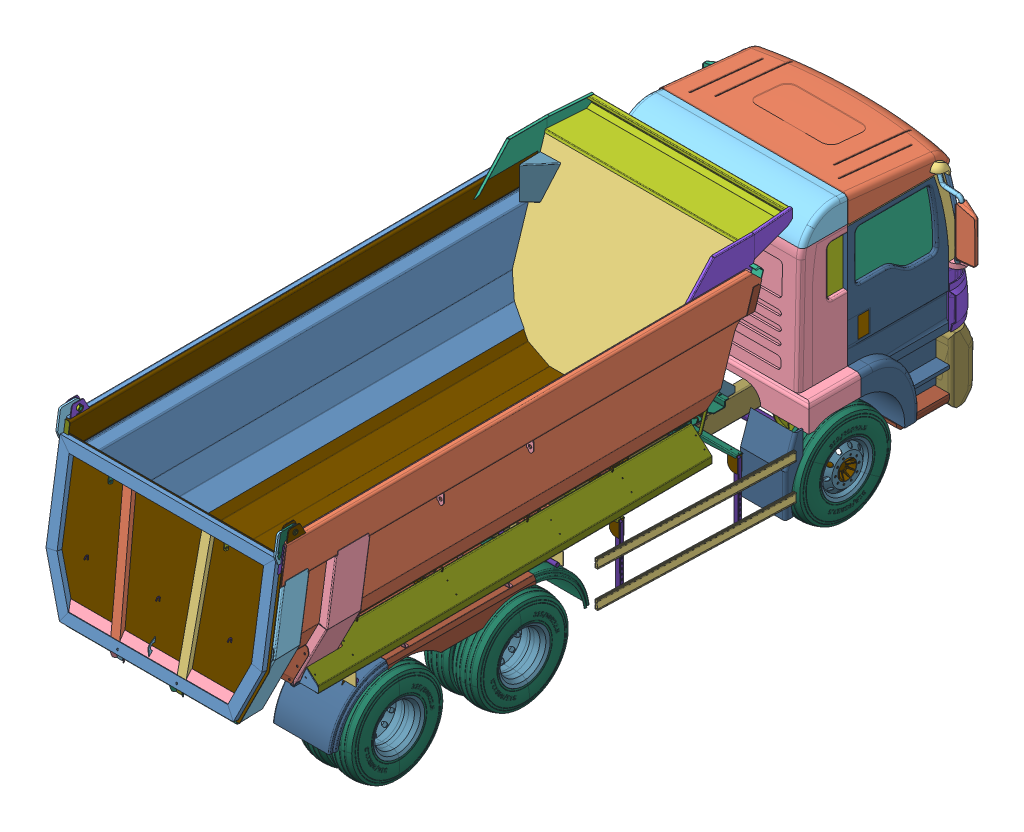
SolidWorks assembly MAN5, configuration Default. Lengths in mm. (continued)
Components (placement in the parent): (continued)
- MAN5.IGS-1: MAN5.IGS [Default] at origin size (3197.79 4674.46 9356.54) (continued)
  - Aynalama33360_pulll.IGS-9: Aynalama33360_pulll.IGS [Default] at (-450.3476 1324.558 3301.5348) x (-0.95234 0 -0.30504) z (0 -1 0) size (40 76.01 3.01)
  - Aynalama33360_pulll.IGS-10: Aynalama33360_pulll.IGS [Default] at (-450.3476 1352.558 3301.5348) x (-0.995286 0 0.096983) z (0 -1 0) size (40 76.01 3.01)
  - Aynalama33360_pulll.IGS-11: Aynalama33360_pulll.IGS [Default] at (-444.4001 1395.558 3378.3048) x (0.404503 0 -0.914537) z (0 -1 0) size (40 76.01 3.01)
  - Aynalama33360_pulll.IGS-12: Aynalama33360_pulll.IGS [Default] at (-450.3476 1395.558 3301.5348) x (0.404503 0 -0.914537) z (0 -1 0) size (40 76.01 3.01)
  - Aynalama33360_esnek baglanti poliuretan takoz.IGS-1: Aynalama33360_esnek baglanti poliuretan takoz.IGS [Default] at (-479.517 1445.558 2461.1366) x (0.305771 0 -0.952105) z (-0.952105 0 -0.305771) size (40.39 40.39 40.78)
  - Aynalama33360_esnek baglanti poliuretan takoz.IGS-2: Aynalama33360_esnek baglanti poliuretan takoz.IGS [Default] at (-479.517 1445.558 2381.1366) x (0.305771 0 -0.952105) z (-0.952105 0 -0.305771) size (40.39 40.39 40.78)
  - Aynalama33360_HEX NUT - ISO 8673 - M16 X 1.5.IGS-1: Aynalama33360_HEX NUT - ISO 8673 - M16 X 1.5.IGS [Default] at (-479.517 1463.358 2461.1366) x (0 -1 0) z (-0.270173 0 -0.962812) size (15.03 27.75 27.75)
  - Aynalama33360_HEX NUT - ISO 8673 - M16 X 1.5.IGS-2: Aynalama33360_HEX NUT - ISO 8673 - M16 X 1.5.IGS [Default] at (-479.517 1463.358 2381.1366) x (0 -1 0) z (-0.270173 0 -0.962812) size (15.03 27.75 27.75)
  - Aynalama33360_HEX NUT - ISO 8673 - M16 X 1.5.IGS-3: Aynalama33360_HEX NUT - ISO 8673 - M16 X 1.5.IGS [Default] at (-444.4001 1413.358 3378.3048) x (0 -1 0) z (0.336021 0 -0.941854) size (15.03 27.75 27.75)
  - Aynalama33360_HEX NUT - ISO 8673 - M16 X 1.5.IGS-4: Aynalama33360_HEX NUT - ISO 8673 - M16 X 1.5.IGS [Default] at (-450.3476 1413.358 3301.5348) x (0 -1 0) z (0.336021 0 -0.941854) size (15.03 27.75 27.75)
  - Aynalama33360_MS 008.IGS-1: Aynalama33360_MS 008.IGS [Default] at (-609.242 1337.558 3134.9181) x (0.077241 0 0.997012) z (0 1 0) size (151.36 57.01 58.73)
  - Aynalama33360_MS 009.IGS-1: Aynalama33360_MS 009.IGS [Default] at (-439.052 1337.558 3121.7331) x (-0.077241 0 -0.997012) z (-0.997012 0 0.077241) size (152.03 59.04 8.35)
  - Aynalama33360_burçlu baðlantý burcu.IGS-1: Aynalama33360_burçlu baðlantý burcu.IGS [Default] at (-444.4001 1355.558 3378.3048) x (0.984937 0 0.172914) z (0 -1 0) size (42 42 40.39)
  - Aynalama33360_burçlu baðlantý burcu.IGS-2: Aynalama33360_burçlu baðlantý burcu.IGS [Default] at (-450.3476 1355.558 3301.5348) x (0.984937 0 0.172914) z (0 -1 0) size (42 42 40.39)
  - AynalamaSon_model_3.IGS-1: AynalamaSon_model_3.IGS [Default] at (-365.1668 1272.558 4408.28) x (0 0 -1) z (1 0 0) size (155.01 200.01 10.01)
  - AynalamaSon_model_3.IGS-2: AynalamaSon_model_3.IGS [Default] at (-365.1668 1272.558 5438.28) x (0 0 -1) z (1 0 0) size (155.01 200.01 10.01)
  - AynalamaSon_model_3.IGS-3: AynalamaSon_model_3.IGS [Default] at (-365.1668 1272.558 6138.28) x (0 0 -1) z (1 0 0) size (155.01 200.01 10.01)
  - Aynalama33360_arkamilbaðlantý.IGS-1: Aynalama33360_arkamilbaðlantý.IGS [Default] at (-365.1668 311.3597 8865.1072) x (0 0 -1) z (1 0 0) size (490.66 250.98 10.19)
  - Ayak U þase parçasý.IGS-1: Ayak U þase parçasý.IGS [Default] at (-372.5244 1364.558 6412.1883) x (1 0 0) z (0 1 0) size (60.01 150.01 180.01)
  - Ayak U þase parçasý.IGS-2: Ayak U þase parçasý.IGS [Default] at (-372.5244 1364.558 5250.1883) x (1 0 0) z (0 1 0) size (60.01 150.01 180.01)
  - ayakl flans.IGS-1: ayakl flans.IGS [Default] at (-415.1668 1481.9529 6462.5787) x (0 0 -1) z (1 0 0) size (125.01 130.01 8.01)
  - ayakl flans.IGS-2: ayakl flans.IGS [Default] at (-415.1668 1481.9529 5300.5787) x (0 0 -1) z (1 0 0) size (125.01 130.01 8.01)
  - Üst kapama L ayak sasi parçasý 21.IGS-1: Üst kapama L ayak sasi parçasý 21.IGS [Default] at (-423.1668 1470.1164 6419.9663) x (0 0 1) z (-1 0 0) size (70.01 70.39 760.39)
  - Üst kapama L ayak sasi parçasý 21.IGS-2: Üst kapama L ayak sasi parçasý 21.IGS [Default] at (-423.1668 1470.1164 5257.9663) x (0 0 1) z (-1 0 0) size (70.01 70.39 760.39)
  - Plastik çamurluk üst kapama1.IGS-1: Plastik çamurluk üst kapama1.IGS [Default] at (-520.1668 1374.558 6658.78) x (-1 0 0) z (0 0 -1) size (690.02 215.03 1650.01)
  - YAPI_plastik camurluk.IGS-1: YAPI_plastik camurluk.IGS [Default] at (-530.1668 -54790.0929 231516.4576) x (0 0.148915 -0.98885) z (1 0 0) size (762.44 555.79 670.01)
  - YAPI_boruu.IGS-1: YAPI_boruu.IGS [Default] at (-355.1668 1394.078 6953.9165) x (0 0.37163 0.928381) z (-1 0 0) size (42.01 42.01 802.01)
  - YAPI_plastik cmurluk bru ust bayrak.IGS-1: YAPI_plastik cmurluk bru ust bayrak.IGS [Default] at (-1051.5754 -129957.1173 197509.9483) x (0 0.487288 -0.873241) z (1 0 0) size (168.01 58.89 5.62)
  - YAPI_plastik cmurluk bru ust bayrak.IGS-2: YAPI_plastik cmurluk bru ust bayrak.IGS [Default] at (-751.5754 -129957.1173 197509.9483) x (0 0.487288 -0.873241) z (1 0 0) size (168.01 58.89 5.62)
  - AynalamaYAPI_boruu.IGS-1: AynalamaYAPI_boruu.IGS [Default] at (-355.1668 1394.078 4713.6435) x (0 0.37163 -0.928381) z (1 0 0) size (42.01 42.01 802.01)
  - AynalamaYAPI_boruu.IGS-2: AynalamaYAPI_boruu.IGS [Default] at (406.8332 1394.078 6953.9165) x (0 0.37163 0.928381) z (-1 0 0) size (42.01 42.01 802.01)
  - AynalamaYAPI_plastik cmurluk bru ust bayrak.IGS-1: AynalamaYAPI_plastik cmurluk bru ust bayrak.IGS [Default] at (-1051.5754 -129957.1173 -185842.3882) x (0 0.487288 0.873241) z (-1 0 0) size (168.01 58.28 5.3)
  - AynalamaYAPI_plastik cmurluk bru ust bayrak.IGS-2: AynalamaYAPI_plastik cmurluk bru ust bayrak.IGS [Default] at (-751.5754 -129957.1173 -185842.3882) x (0 0.487288 0.873241) z (-1 0 0) size (168.01 58.28 5.3)
  - AynalamaYAPI_plastik cmurluk bru ust bayrak.IGS-3: AynalamaYAPI_plastik cmurluk bru ust bayrak.IGS [Default] at (803.2418 -129957.1173 197509.9483) x (0 0.487288 -0.873241) z (1 0 0) size (168.01 58.28 5.3)
  - AynalamaYAPI_plastik cmurluk bru ust bayrak.IGS-4: AynalamaYAPI_plastik cmurluk bru ust bayrak.IGS [Default] at (1103.2418 -129957.1173 197509.9483) x (0 0.487288 -0.873241) z (1 0 0) size (168.01 58.28 5.3)
  - AynalamaYAPI_plastik camurluk.IGS-1: AynalamaYAPI_plastik camurluk.IGS [Default] at (-530.1668 -54790.0929 -219848.8976) x (0 0.148915 0.98885) z (-1 0 0) size (762.44 554.71 670.01)
  - AynalamaYAPI_plastik camurluk.IGS-2: AynalamaYAPI_plastik camurluk.IGS [Default] at (581.8332 -54790.0929 231516.4576) x (0 0.148915 -0.98885) z (1 0 0) size (762.44 554.71 670.01)
  - AynalamaPlastik çamurluk üst kapama1.IGS-1: AynalamaPlastik çamurluk üst kapama1.IGS [Default] at (571.8332 1374.558 6658.78) size (690.02 215.03 1650.01)
  - Aynalamaayakl flans.IGS-1: Aynalamaayakl flans.IGS [Default] at (466.8332 1481.9529 6462.5787) x (0 0 -1) z (1 0 0) size (125.01 130.01 8.01)
  - Aynalamaayakl flans.IGS-2: Aynalamaayakl flans.IGS [Default] at (466.8332 1481.9529 5300.5787) x (0 0 -1) z (1 0 0) size (125.01 130.01 8.01)
  - AynalamaÜst kapama L ayak sasi parçasý 21.IGS-1: AynalamaÜst kapama L ayak sasi parçasý 21.IGS [Default] at (474.8332 1470.1164 6419.9663) x (0 0 1) z (-1 0 0) size (70.01 70.39 760.39)
  - AynalamaÜst kapama L ayak sasi parçasý 21.IGS-2: AynalamaÜst kapama L ayak sasi parçasý 21.IGS [Default] at (474.8332 1470.1164 5257.9663) x (0 0 1) z (-1 0 0) size (70.01 70.39 760.39)
  - AynalamaAyak U þase parçasý.IGS-1: AynalamaAyak U þase parçasý.IGS [Default] at (424.1908 1364.558 6412.1883) x (-1 0 0) z (0 -1 0) size (60.01 150.01 180.01)
  - AynalamaAyak U þase parçasý.IGS-2: AynalamaAyak U þase parçasý.IGS [Default] at (424.1908 1364.558 5250.1883) x (-1 0 0) z (0 -1 0) size (60.01 150.01 180.01)
  - AynalamaAynalamaYAPI_plastik camurluk.IGS-1: AynalamaAynalamaYAPI_plastik camurluk.IGS [Default] at (581.8332 -54790.0929 -219848.8976) x (0 0.148915 0.98885) z (-1 0 0) size (762.44 555.79 670.01)
  - AynalamaAynalamaYAPI_plastik cmurluk bru ust bayrak.IGS-1: AynalamaAynalamaYAPI_plastik cmurluk bru ust bayrak.IGS [Default] at (803.2418 -129957.1173 -185842.3882) x (0 0.487288 0.873241) z (-1 0 0) size (168.01 58.89 5.62)
  - AynalamaAynalamaYAPI_plastik cmurluk bru ust bayrak.IGS-2: AynalamaAynalamaYAPI_plastik cmurluk bru ust bayrak.IGS [Default] at (1103.2418 -129957.1173 -185842.3882) x (0 0.487288 0.873241) z (-1 0 0) size (168.01 58.89 5.62)
  - AynalamaAynalamaYAPI_boruu.IGS-1: AynalamaAynalamaYAPI_boruu.IGS [Default] at (406.8332 1394.078 4713.6435) x (0 0.37163 -0.928381) z (1 0 0) size (42.01 42.01 802.01)
  - M5 - erp33360_TABAN 8 MM ST.IGS-1: M5 - erp33360_TABAN 8 MM ST.IGS [Default] at (2711.0125 794.7914 10334.4906) x (-1 0 0) z (0 0.005539 -0.999985) size (1888.79 207.2 5094.21)
  - M5 - erp33360_YAN 6 MM ST.IGS-1: M5 - erp33360_YAN 6 MM ST.IGS [Default] at (-3149.2259 1030.8858 2339.3517) x (1 0 0) z (0 -0.005539 0.999985) size (345.97 1417.88 5529.51)
  - M5 - erp33360_MirrorYAN 6 MM ST.IGS-1: M5 - erp33360_MirrorYAN 6 MM ST.IGS [Default] at (-555.1726 1030.8858 2339.3517) x (1 0 0) z (0 -0.005539 0.999985) size (345.97 1417.88 5529.51)
  - M5 - erp33360_ÖNPANEL 6 MM ST.IGS-1: M5 - erp33360_ÖNPANEL 6 MM ST.IGS [Default] at (3482.8014 -1032.9201 3905.3475) x (-1 0 0) z (0 -0.303745 -0.952753) size (2308.01 1803.01 6.01)
  - M5 - erp33360_ÖZBEKÝSTAN kulak krosu.IGS-1: M5 - erp33360_ÖZBEKÝSTAN kulak krosu.IGS [Default] at (1008.3381 57456.9661 -197352.5561) x (0 -0.005539 0.999985) z (-1 0 0) size (380.01 85.01 1965.01)
  - M5 - erp33360_ÖZBEKÝSTAN Büyük Yan Kros.IGS-1: M5 - erp33360_ÖZBEKÝSTAN Büyük Yan Kros.IGS [Default] at (-1441.0535 2620.6295 10762.7624) x (0.390684 -0.920485 0.00854) z (-0.920505 -0.39072 -0.00295) size (1326.04 856.53 453.89)
  - M5 - erp33360_ÖZBEKÝSTAN En Arka Taban Krosu.IGS-1: M5 - erp33360_ÖZBEKÝSTAN En Arka Taban Krosu.IGS [Default] at (1075.8381 60014.1611 -302542.0948) x (0 -0.005539 0.999985) z (-1 0 0) size (149.44 170.01 1920.62)
  - M5 - erp33360_ÖZBEKÝSTAN küçük yan kros.IGS-1: M5 - erp33360_ÖZBEKÝSTAN küçük yan kros.IGS [Default] at (-1242.2043 1026.8349 7834.3506) x (0 0.150962 0.98854) z (0 0.98854 -0.150962) size (819.28 418.27 1464.92)
  - M5 - erp33360_HD_601.IGS-1: M5 - erp33360_HD_601.IGS [Default] at (25.8154 3173.364 2552.8076) x (1 -0.000135 0.000043) z (0.000141 0.952753 -0.303745) size (240.01 5.01 319.27)
  - M5 - erp33360_HD_602.IGS-1: M5 - erp33360_HD_602.IGS [Default] at (21.8458 3335.9395 2354.6947) x (-0.000135 -0.999999 -0.001661) z (1 -0.000135 0.000043) size (8.01 308.36 252.01)
  - M5 - erp33360_KMK 214.IGS-1: M5 - erp33360_KMK 214.IGS [Default] at (-94.1776 3178.3559 2403.4311) x (-0.000135 -0.999999 -0.001661) z (1 -0.000135 0.000043) size (302.82 405.21 6.16)
  - M5 - erp33360_KMK 214.IGS-2: M5 - erp33360_KMK 214.IGS [Default] at (151.8224 3178.3227 2403.4417) x (-0.000135 -0.999999 -0.001661) z (1 -0.000135 0.000043) size (302.82 405.21 6.16)
  - M5 - erp33360_HD_604.IGS-1: M5 - erp33360_HD_604.IGS [Default] at (-16.9955 -12880.7962 5963.2245) x (-0.000135 -0.999959 0.009015) z (1 -0.000135 0.000043) size (157.84 185.04 79.51)
  - M5 - erp33360_HD_604.IGS-2: M5 - erp33360_HD_604.IGS [Default] at (143.5045 -12880.8178 5963.2314) x (-0.000135 -0.999959 0.009015) z (1 -0.000135 0.000043) size (157.84 185.04 79.51)
  - M5 - erp33360_KMK 213.IGS-1: M5 - erp33360_KMK 213.IGS [Default] at (-6.6689 3239.4117 2394.0646) x (0.000135 0.999992 0.003883) z (-1 0.000135 -0.000043) size (167.21 326.2 8.85)
  - M5 - erp33360_KMK 213.IGS-2: M5 - erp33360_KMK 213.IGS [Default] at (66.3311 3239.4018 2394.0677) x (0.000135 0.999992 0.003883) z (-1 0.000135 -0.000043) size (167.21 326.2 8.85)
  - M5 - erp33360_HDS_606.IGS-1: M5 - erp33360_HDS_606.IGS [Default] at (-44.6627 3267.742 2337.2221) x (-0.000007 0.253545 0.967324) z (1 -0.000135 0.000043) size (72.14 72 30.01)
  - M5 - erp33360_HDS_607.IGS-1: M5 - erp33360_HDS_607.IGS [Default] at (66.3373 3267.7271 2337.2269) x (-0.000135 -0.999999 -0.001661) z (1 -0.000135 0.000043) size (72 72 10.01)
  - M5 - erp33360_HDS_608.IGS-1: M5 - erp33360_HDS_608.IGS [Default] at (-50.6627 3267.7428 2337.2219) x (-0.000141 -0.967324 0.253545) z (1 -0.000135 0.000043) size (49 49.59 145.46)
  - M5 - erp33360_ÖZBEKÝSTAN ön dikme.IGS-1: M5 - erp33360_ÖZBEKÝSTAN ön dikme.IGS [Default] at (-168195.7295 -7372.7682 -32398.8379) x (1 0 0) z (0 -0.952753 0.303745) size (152.43 80.67 1836.48)
  - M5 - erp33360_ÖZBEKÝSTAN öngöðüs kuþak krosu.IGS-1: M5 - erp33360_ÖZBEKÝSTAN öngöðüs kuþak krosu.IGS [Default] at (-1218.0423 -352742.0932 105385.5445) x (0 0.953195 -0.302356) z (1 0 0) size (367.53 86.57 1008.59)
  - M5 - erp33360_iç kayýtr.IGS-1: M5 - erp33360_iç kayýtr.IGS [Default] at (-3031.6176 2222.8106 2486.7487) x (1 0 0) z (0 -0.005539 0.999985) size (71.18 295.53 5329.09)
  - M5 - erp33360_ÖZBEKÝSTAN kilit krosu bayrak.IGS-1: M5 - erp33360_ÖZBEKÝSTAN kilit krosu bayrak.IGS [Default] at (-4536.9786 -10452.359 13580.8312) x (1 0 0) z (0 0.430757 0.902468) size (617.2 521.07 142.75)
  - M5 - erp33360_ÖZBEKÝSTAN kilit takviye 2.IGS-1: M5 - erp33360_ÖZBEKÝSTAN kilit takviye 2.IGS [Default] at (-236.4961 1585.2287 7897.2862) x (1 0 0) z (0 -0.144581 -0.989493) size (437.72 186.93 142.51)
  - M5 - erp33360_MirrorÖZBEKÝSTAN ön dikme.IGS-1: M5 - erp33360_MirrorÖZBEKÝSTAN ön dikme.IGS [Default] at (164491.3309 -7373.2589 -32402.351) x (1 0 0) z (0 -0.952753 0.303745) size (152.47 80.67 1836.48)
  - M5 - erp33360_MirrorÖZBEKÝSTAN Büyük Yan Kros.IGS-1: M5 - erp33360_MirrorÖZBEKÝSTAN Büyük Yan Kros.IGS [Default] at (25.2904 -837.5574 10794.8351) x (0.390684 0.920485 -0.00854) z (0.920505 -0.39072 -0.00295) size (1326.07 873.47 448.36)
  - M5 - erp33360_AynalamaÖZBEKÝSTAN kilit krosu bayrak.IGS-1: M5 - erp33360_AynalamaÖZBEKÝSTAN kilit krosu bayrak.IGS [Default] at (4588.6547 -10452.359 13580.8312) x (-1 0 0) z (0 -0.430757 -0.902468) size (617.2 521.07 142.75)
  - M5 - erp33360_çamurluk sacý_k4.IGS-1: M5 - erp33360_çamurluk sacý_k4.IGS [Default] at (-3152.8435 697.3199 3027.2234) x (0.999992 0.00393 0.000022) z (0 -0.005539 0.999985) size (264.76 280.89 4405.19)
  - M5 - erp33360_ön çamurluk ayaðý_k6.IGS-1: M5 - erp33360_ön çamurluk ayaðý_k6.IGS [Default] at (-2993.8042 653.5355 3032.9809) x (0.999992 0.003934 0.000022) z (0 -0.005539 0.999985) size (508.17 269.14 291.41)
  - M5 - erp33360_iç çamurluk ayaðý_k6.IGS-1: M5 - erp33360_iç çamurluk ayaðý_k6.IGS [Default] at (-2594.5939 882.7123 5853.2935) x (0.999992 0.003934 0.000022) z (0 -0.005539 0.999985) size (492.87 198.39 270.05)
  - M5 - erp33360_iç çamurluk ayaðý_k6.IGS-2: M5 - erp33360_iç çamurluk ayaðý_k6.IGS [Default] at (-2594.5941 893.5402 3898.3234) x (0.999992 0.003934 0.000022) z (0 -0.005539 0.999985) size (492.87 198.39 270.05)
  - M5 - erp33360_arka çamurluk ayaðý_6mm.IGS-1: M5 - erp33360_arka çamurluk ayaðý_6mm.IGS [Default] at (-2965.4571 531.7536 7416.3737) x (0.999992 0.003934 0.000022) z (0 -0.005539 0.999985) size (216.15 187.55 190)
  - M5 - erp33360_iç çamurluk ayaðý_paspas gelenler__.IGS-1: M5 - erp33360_iç çamurluk ayaðý_paspas gelenler__.IGS [Default] at (-2594.5513 889.1528 4697.3114) x (0.999992 0.003934 0.000022) z (0 -0.005539 0.999985) size (492.87 225.4 270.05)
  - M5 - erp33360_iç çamurluk ayaðý_paspas gelenler__.IGS-2: M5 - erp33360_iç çamurluk ayaðý_paspas gelenler__.IGS [Default] at (-2594.5511 876.3532 7008.276) x (0.999992 0.003934 0.000022) z (0 -0.005539 0.999985) size (492.87 225.4 270.05)
  - M5 - erp33360_KMK 236.IGS-1: M5 - erp33360_KMK 236.IGS [Default] at (-21515.7908 1653.5699 -20713.8331) x (-1 0 0) z (0 -0.999985 -0.005539) size (250.01 390.01 12.01)
  - M5 - erp33360_KMS 202.IGS-1: M5 - erp33360_KMS 202.IGS [Default] at (-434.1619 1492.1837 7160.4219) x (0 -0.999985 -0.005539) z (0 -0.005539 0.999985) size (60.01 45.01 8.01)
  - M5 - erp33360_KMS 202.IGS-2: M5 - erp33360_KMS 202.IGS [Default] at (-434.1619 1490.9985 7374.4186) x (0 -0.999985 -0.005539) z (0 -0.005539 0.999985) size (60.01 45.01 8.01)
  - M5 - erp33360_KMS 202.IGS-3: M5 - erp33360_KMS 202.IGS [Default] at (-564.1619 1492.1394 7168.4218) x (0 -0.999985 -0.005539) z (0 0.005539 -0.999985) size (60.01 45.01 8.01)
  - M5 - erp33360_KMS 202.IGS-4: M5 - erp33360_KMS 202.IGS [Default] at (-564.1619 1490.9542 7382.4185) x (0 -0.999985 -0.005539) z (0 0.005539 -0.999985) size (60.01 45.01 8.01)
  - M5 - erp33360_HD 654.IGS-1: M5 - erp33360_HD 654.IGS [Default] at (-404.1619 1405.558 7270.78) x (-1 0 0) z (0 0.1474 -0.989077) size (171.89 100 100)
  - M5 - erp33360_KMK 226.IGS-1: M5 - erp33360_KMK 226.IGS [Default] at (-579.1619 1577.7689 7055.8305) x (0 -0.005539 0.999985) z (1 0 0) size (86.06 24.53 5.01)
  - M5 - erp33360_KMS 298.IGS-1: M5 - erp33360_KMS 298.IGS [Default] at (-564.1619 -80578.3775 132955.5354) x (0 -0.006857 0.999976) z (1 0 0) size (380.01 164.01 10.01)
  - M5 - erp33360_KMS 298.IGS-2: M5 - erp33360_KMS 298.IGS [Default] at (-444.1619 -80578.3775 132955.5354) x (0 -0.006857 0.999976) z (1 0 0) size (380.01 164.01 10.01)
  - M5 - erp33360_KMS 207.IGS-1: M5 - erp33360_KMS 207.IGS [Default] at (-554.1619 30316.5861 -13567.0822) x (0 0.005539 -0.999985) z (1 0 0) size (344.29 150.76 110.01)
  - M5 - erp33360_kros köþebent.IGS-1: M5 - erp33360_kros köþebent.IGS [Default] at (-937.9193 1507.0066 7461.4935) x (-0.390731 0.920493 0.004765) z (0.000854 0.005539 -0.999984) size (60.24 41.83 380.01)
  - M5 - erp33360_Aynalamaçamurluk ayaðý köþebenti_6mm.IGS-1: M5 - erp33360_Aynalamaçamurluk ayaðý köþebenti_6mm.IGS [Default] at (-3118.1274 743.529 5840.5224) x (1 0 0) z (0 -0.005539 0.999985) size (278.76 183.65 137.55)
  - M5 - erp33360_Aynalamaçamurluk ayaðý köþebenti_6mm.IGS-2: M5 - erp33360_Aynalamaçamurluk ayaðý köþebenti_6mm.IGS [Default] at (-3118.1274 749.9315 4684.5402) x (1 0 0) z (0 -0.005539 0.999985) size (278.76 183.65 137.55)
  - M5 - erp33360_Aynalamaçamurluk ayaðý köþebenti_6mm.IGS-3: M5 - erp33360_Aynalamaçamurluk ayaðý köþebenti_6mm.IGS [Default] at (-3118.1274 737.132 6995.5047) x (1 0 0) z (0 -0.005539 0.999985) size (278.76 183.65 137.55)
  - M5 - erp33360_Aynalamaçamurluk ayaðý köþebenti_6mm.IGS-4: M5 - erp33360_Aynalamaçamurluk ayaðý köþebenti_6mm.IGS [Default] at (-3118.1274 754.3568 3885.5524) x (1 0 0) z (0 -0.005539 0.999985) size (278.76 183.65 137.55)
  - M5 - erp33360_çamurluk ayaðý küçük köþebent 6mm.IGS-1: M5 - erp33360_çamurluk ayaðý küçük köþebent 6mm.IGS [Default] at (-998.8645 -778.8309 7396.4339) x (-0.39073 0.920491 0.005098) z (0.000724 0.005846 -0.999983) size (119.97 59.66 44.44)
  - M5 - erp33360_þase kaçmazý 6 mm.IGS-1: M5 - erp33360_þase kaçmazý 6 mm.IGS [Default] at (-2259.5031 543.4533 3492.8973) x (0.996972 0.000431 -0.077762) z (0.077763 -0.005522 0.996957) size (80.34 92.23 6.28)
  - M5 - erp33360_þase kaçmazý 6 mm.IGS-2: M5 - erp33360_þase kaçmazý 6 mm.IGS [Default] at (-2265.2576 543.8619 3419.1225) x (0.996972 0.000431 -0.077762) z (0.077763 -0.005522 0.996957) size (80.34 92.23 6.28)
  - M5 - erp33360_þase kaçmazý arka sacý_6mm.IGS-1: M5 - erp33360_þase kaçmazý arka sacý_6mm.IGS [Default] at (-2258.7255 543.3981 3502.8668) x (0.996972 0.000431 -0.077762) z (0.077763 -0.005522 0.996957) size (89.64 108.39 102.98)
  - M5 - erp33360_Aynalamaiç kayýtr.IGS-1: M5 - erp33360_Aynalamaiç kayýtr.IGS [Default] at (3083.2937 2222.8106 2486.7487) x (-1 0 0) z (0 0.005539 -0.999985) size (71.18 295.53 5329.09)
  - M5 - erp33360_çamurluk ayaðý köþebenti_6mm.IGS-1: M5 - erp33360_çamurluk ayaðý köþebenti_6mm.IGS [Default] at (-3118.1274 759.0424 3039.5654) x (1 0 0) z (0 -0.005539 0.999985) size (276.76 187.48 132.2)
  - M5 - erp33360_siperlik yan sacý.IGS-1: M5 - erp33360_siperlik yan sacý.IGS [Default] at (-1128.1619 2915.0348 3291.601) x (0 0.005539 -0.999985) z (1 0 0) size (1286.13 449.51 548.53)
  - M5 - erp33360_siperlik.IGS-1: M5 - erp33360_siperlik.IGS [Default] at (-1128.1619 3194.9843 2755.6366) x (0 0.005539 -0.999985) z (1 0 0) size (492.33 158.99 2308.01)
  - M5 - erp33360_Aynalamasiperlik yan sacý.IGS-1: M5 - erp33360_Aynalamasiperlik yan sacý.IGS [Default] at (1179.8381 2915.0348 3291.601) x (0 0.005539 -0.999985) z (1 0 0) size (1286.13 442.38 555.99)
  - M5 - erp33360_Ön arka çamurluk_Yeni Tip_k3.IGS-1: M5 - erp33360_Ön arka çamurluk_Yeni Tip_k3.IGS [Default] at (-597.7041 1563.9747 4685.8761) x (0 -0.005539 0.999985) z (-0.999995 -0.003098 -0.000017) size (3.1 205.01 600.01)
  - M5 - erp33360_Ön arka çamurluk_Yeni Tip_k3.IGS-2: M5 - erp33360_Ön arka çamurluk_Yeni Tip_k3.IGS [Default] at (-597.7039 1551.1751 6996.8407) x (0 -0.005539 0.999985) z (-0.999995 -0.003098 -0.000017) size (3.1 205.01 600.01)
  - M5 - erp33360_önpanel dýþköþe takviyesi.IGS-1: M5 - erp33360_önpanel dýþköþe takviyesi.IGS [Default] at (-1224.329 2619.4628 2447.6999) x (0 0.302356 0.953195) z (-1 0 0) size (89.64 267.98 79.8)
  - M5 - erp33360_Aynalamaönpanel dýþköþe takviyesi.IGS-1: M5 - erp33360_Aynalamaönpanel dýþköþe takviyesi.IGS [Default] at (1276.0051 2619.4628 2447.6999) x (0 0.302356 0.953195) z (-1 0 0) size (89.64 267.98 79.8)
  - M5 - erp33360_iç sehim takviyesi.IGS-1: M5 - erp33360_iç sehim takviyesi.IGS [Default] at (-384.1619 1408.1547 7304.7483) x (0 0.005539 -0.999985) z (1 0 0) size (146.01 77.01 820.01)
  - M5 - erp33360_iç sehim takviyesi.IGS-2: M5 - erp33360_iç sehim takviyesi.IGS [Default] at (435.8381 1408.529 7237.1701) x (0 -0.005539 0.999985) z (-1 0 0) size (146.01 77.01 820.01)
  - M5 - erp33360_önpanel içköþe takviyesi.IGS-1: M5 - erp33360_önpanel içköþe takviyesi.IGS [Default] at (1251.1068 2575.8808 2876.615) x (-0.69944 0.002869 -0.714686) z (0.714692 0.002808 -0.699434) size (328.95 380.59 175.4)
  - M5 - erpAynalama33360_önpanel içköþe takviyesi.IGS-1: M5 - erpAynalama33360_önpanel içköþe takviyesi.IGS [Default] at (-1199.4307 2575.8808 2876.615) x (0.69944 0.002869 -0.714686) z (0.714692 -0.002808 0.699434) size (328.95 380.59 181.53)
  - M5 - erp33360_siperlik lamasý.IGS-1: M5 - erp33360_siperlik lamasý.IGS [Default] at (-1128.1619 2713.3631 2659.0764) x (-1 0 0) z (0 -0.30377 -0.952745) size (29.96 171.79 4.01)
  - M5 - erpAynalama33360_çamurluk sacý_k4.IGS-1: M5 - erpAynalama33360_çamurluk sacý_k4.IGS [Default] at (3204.5196 697.3199 3027.2234) x (-0.999992 0.00393 0.000022) z (0 0.005539 -0.999985) size (264.76 280.89 4405.19)
  - M5 - erpAynalama33360_ön çamurluk ayaðý_k6.IGS-1: M5 - erpAynalama33360_ön çamurluk ayaðý_k6.IGS [Default] at (3045.4803 653.5355 3032.9809) x (-0.999992 0.003934 0.000022) z (0 0.005539 -0.999985) size (507.88 268.85 302.92)
  - M5 - erpAynalama33360_iç çamurluk ayaðý_k6.IGS-1: M5 - erpAynalama33360_iç çamurluk ayaðý_k6.IGS [Default] at (2646.27 882.7123 5853.2935) x (-0.999992 0.003934 0.000022) z (0 0.005539 -0.999985) size (492.69 198.39 258.62)
  - M5 - erpAynalama33360_iç çamurluk ayaðý_k6.IGS-2: M5 - erpAynalama33360_iç çamurluk ayaðý_k6.IGS [Default] at (2646.2702 893.5402 3898.3234) x (-0.999992 0.003934 0.000022) z (0 0.005539 -0.999985) size (492.69 198.39 258.62)
  - M5 - erpAynalama33360_arka çamurluk ayaðý_6mm.IGS-1: M5 - erpAynalama33360_arka çamurluk ayaðý_6mm.IGS [Default] at (3017.1332 531.7536 7416.3737) x (-0.999992 0.003934 0.000022) z (0 0.005539 -0.999985) size (216.15 187.26 178.81)
  - M5 - erpAynalama33360_iç çamurluk ayaðý_paspas gelenler__.IGS-1: M5 - erpAynalama33360_iç çamurluk ayaðý_paspas gelenler__.IGS [Default] at (2646.2274 889.1528 4697.3114) x (-0.999992 0.003934 0.000022) z (0 0.005539 -0.999985) size (492.69 225.4 258.62)
  - M5 - erpAynalama33360_iç çamurluk ayaðý_paspas gelenler__.IGS-2: M5 - erpAynalama33360_iç çamurluk ayaðý_paspas gelenler__.IGS [Default] at (2646.2272 876.3532 7008.276) x (-0.999992 0.003934 0.000022) z (0 0.005539 -0.999985) size (492.69 225.4 258.62)
  - M5 - erpAynalama33360_Ön arka çamurluk_Yeni Tip_k3.IGS-1: M5 - erpAynalama33360_Ön arka çamurluk_Yeni Tip_k3.IGS [Default] at (649.3802 1563.9747 4685.8761) x (0 -0.005539 0.999985) z (-0.999995 0.003098 0.000017) size (3.07 205.01 600.01)
  - M5 - erpAynalama33360_Ön arka çamurluk_Yeni Tip_k3.IGS-2: M5 - erpAynalama33360_Ön arka çamurluk_Yeni Tip_k3.IGS [Default] at (649.38 1551.1751 6996.8407) x (0 -0.005539 0.999985) z (-0.999995 0.003098 0.000017) size (3.07 205.01 600.01)
  - M5 - erpAynalama33360_KMK 236.IGS-1: M5 - erpAynalama33360_KMK 236.IGS [Default] at (21567.4669 1653.5699 -20713.8331) x (1 0 0) z (0 0.999985 0.005539) size (250.01 390.01 12.01)
  - M5 - erpAynalama33360_KMS 202.IGS-1: M5 - erpAynalama33360_KMS 202.IGS [Default] at (485.8381 1492.1837 7160.4219) x (0 -0.999985 -0.005539) z (0 0.005539 -0.999985) size (60.01 45.01 8.01)
  - M5 - erpAynalama33360_KMS 202.IGS-2: M5 - erpAynalama33360_KMS 202.IGS [Default] at (485.8381 1490.9985 7374.4186) x (0 -0.999985 -0.005539) z (0 0.005539 -0.999985) size (60.01 45.01 8.01)
  - M5 - erpAynalama33360_KMS 202.IGS-3: M5 - erpAynalama33360_KMS 202.IGS [Default] at (615.8381 1492.1394 7168.4218) x (0 -0.999985 -0.005539) z (0 -0.005539 0.999985) size (60.01 45.01 8.01)
  - M5 - erpAynalama33360_KMS 202.IGS-4: M5 - erpAynalama33360_KMS 202.IGS [Default] at (615.8381 1490.9542 7382.4185) x (0 -0.999985 -0.005539) z (0 -0.005539 0.999985) size (60.01 45.01 8.01)
  - M5 - erpAynalama33360_HD 654.IGS-1: M5 - erpAynalama33360_HD 654.IGS [Default] at (455.8381 1405.558 7270.78) x (1 0 0) z (0 -0.1474 0.989077) size (170.95 100 100)
  - M5 - erpAynalama33360_KMK 226.IGS-1: M5 - erpAynalama33360_KMK 226.IGS [Default] at (630.8381 1577.7689 7055.8305) x (0 -0.005539 0.999985) z (1 0 0) size (86.06 25.37 5.43)
  - M5 - erpAynalama33360_KMS 298.IGS-1: M5 - erpAynalama33360_KMS 298.IGS [Default] at (615.8381 -80578.3775 132955.5354) x (0 -0.006857 0.999976) z (1 0 0) size (380.01 164.44 10.44)
  - M5 - erpAynalama33360_KMS 298.IGS-2: M5 - erpAynalama33360_KMS 298.IGS [Default] at (495.8381 -80578.3775 132955.5354) x (0 -0.006857 0.999976) z (1 0 0) size (380.01 164.44 10.44)
  - M5 - erpAynalama33360_KMS 207.IGS-1: M5 - erpAynalama33360_KMS 207.IGS [Default] at (605.8381 30316.5861 -13567.0822) x (0 0.005539 -0.999985) z (1 0 0) size (344.29 150.76 110.01)
  - M5 - erpAynalama33360_kros köþebent.IGS-1: M5 - erpAynalama33360_kros köþebent.IGS [Default] at (989.5954 1507.0066 7461.4935) x (0.390731 0.920493 0.004765) z (0.000854 -0.005539 0.999984) size (60.24 41.83 380.01)
  - M5 - erpAynalama33360_Aynalamaçamurluk ayaðý köþebenti_6mm.IGS-1: M5 - erpAynalama33360_Aynalamaçamurluk ayaðý köþebenti_6mm.IGS [Default] at (3169.8035 743.529 5840.5224) x (-1 0 0) z (0 0.005539 -0.999985) size (278.95 183.65 132.2)
  - M5 - erpAynalama33360_Aynalamaçamurluk ayaðý köþebenti_6mm.IGS-2: M5 - erpAynalama33360_Aynalamaçamurluk ayaðý köþebenti_6mm.IGS [Default] at (3169.8035 749.9315 4684.5402) x (-1 0 0) z (0 0.005539 -0.999985) size (278.95 183.65 132.2)
  - M5 - erpAynalama33360_Aynalamaçamurluk ayaðý köþebenti_6mm.IGS-3: M5 - erpAynalama33360_Aynalamaçamurluk ayaðý köþebenti_6mm.IGS [Default] at (3169.8035 754.3568 3885.5524) x (-1 0 0) z (0 0.005539 -0.999985) size (278.95 183.65 132.2)
  - M5 - erpAynalama33360_Aynalamaçamurluk ayaðý köþebenti_6mm.IGS-4: M5 - erpAynalama33360_Aynalamaçamurluk ayaðý köþebenti_6mm.IGS [Default] at (3169.8035 737.132 6995.5047) x (-1 0 0) z (0 0.005539 -0.999985) size (278.95 183.65 132.2)
  - M5 - erpAynalama33360_çamurluk ayaðý küçük köþebent 6mm.IGS-1: M5 - erpAynalama33360_çamurluk ayaðý küçük köþebent 6mm.IGS [Default] at (1050.5406 -778.8309 7396.4339) x (0.39073 0.920491 0.005098) z (0.000724 -0.005846 0.999983) size (119.59 59.47 44.54)
  - M5 - erpAynalama33360_þase kaçmazý 6 mm.IGS-1: M5 - erpAynalama33360_þase kaçmazý 6 mm.IGS [Default] at (2311.1792 543.4533 3492.8973) x (-0.996972 0.000431 -0.077762) z (0.077763 0.005522 -0.996957) size (80.57 92.23 6.26)
  - M5 - erpAynalama33360_þase kaçmazý 6 mm.IGS-2: M5 - erpAynalama33360_þase kaçmazý 6 mm.IGS [Default] at (2316.9337 543.8619 3419.1225) x (-0.996972 0.000431 -0.077762) z (0.077763 0.005522 -0.996957) size (80.57 92.23 6.26)
  - M5 - erpAynalama33360_þase kaçmazý arka sacý_6mm.IGS-1: M5 - erpAynalama33360_þase kaçmazý arka sacý_6mm.IGS [Default] at (2310.4016 543.3981 3502.8668) x (-0.996972 0.000431 -0.077762) z (0.077763 0.005522 -0.996957) size (89.64 108.39 102.98)
  - M5 - erpAynalama33360_çamurluk ayaðý köþebenti_6mm.IGS-1: M5 - erpAynalama33360_çamurluk ayaðý köþebenti_6mm.IGS [Default] at (3169.8035 759.0424 3039.5654) x (-1 0 0) z (0 0.005539 -0.999985) size (276.37 187.36 137.55)
  - M5 - erp33360_içkayýt arka kaama.IGS-1: M5 - erp33360_içkayýt arka kaama.IGS [Default] at (-3031.6176 3039.5767 7835.1615) x (1 0 0) z (0 0.150962 0.98854) size (85.58 301.34 5.41)
  - M5 - erpAynalama33360_içkayýt arka kaama.IGS-1: M5 - erpAynalama33360_içkayýt arka kaama.IGS [Default] at (3083.2937 3039.5767 7835.1615) x (-1 0 0) z (0 -0.150962 -0.98854) size (85.18 300.93 5.01)
  - M5 - erp33360_kapak.IGS-1: M5 - erp33360_kapak.IGS [Default] at (-3149.2259 1787.216 8011.4334) x (1 0 0) z (0 0.150962 0.98854) size (2460.01 1628.01 6.01)
  - M5 - erp33390_kapak npu 120lik.IGS-1: M5 - erp33390_kapak npu 120lik.IGS [Default] at (-3149.2259 1788.1218 8017.3646) x (1 0 0) z (0 0.150962 0.98854) size (2435.1 1598.77 469.96)
  - M5 - erp33360_arka dik npu 100 lük.IGS-1: M5 - erp33360_arka dik npu 100 lük.IGS [Default] at (-294.9512 1616.8559 8137.0224) x (0 0.150962 0.98854) z (-0.99863 -0.051736 0.007901) size (50.01 1376.12 100.01)
  - M5 - erpAynalama33360_arka dik npu 100 lük.IGS-1: M5 - erpAynalama33360_arka dik npu 100 lük.IGS [Default] at (346.6273 1616.8559 8137.0224) x (0 0.150962 0.98854) z (-0.99863 0.051736 -0.007901) size (50.01 1376.12 100.01)
  - M5 - erp33360_Kapak alt kapama.IGS-1: M5 - erp33360_Kapak alt kapama.IGS [Default] at (-1265.0645 1661.7794 8011.9099) x (0 0.58466 0.811278) z (1 0 0) size (5.01 100.01 1854.78)
  - M5 - erptutamak.IGS-1: M5 - erptutamak.IGS [Default] at (21.8381 2040.7142 7665.0258) x (0 -0.917046 0.398782) z (-1 0 0) size (172.85 55.73 8.37)
  - M5 - erp3360_kapak kanca mapasý.IGS-1: M5 - erp3360_kapak kanca mapasý.IGS [Default] at (-615.1383 4085.3577 7694.3682) x (0 -0.150962 -0.98854) z (1 0 0) size (50.49 80.49 8.49)
  - M5 - erpAynalama3360_kapak kanca mapasý.IGS-1: M5 - erpAynalama3360_kapak kanca mapasý.IGS [Default] at (666.8144 4085.3577 7694.3682) x (0 -0.150962 -0.98854) z (1 0 0) size (50.01 80.01 8.01)
  - M5 - erp33360_kilit parçasý ayaðý.IGS-1: M5 - erp33360_kilit parçasý ayaðý.IGS [Default] at (-276.1619 1349.6278 8183.4157) x (0 0.005539 -0.999985) z (1 0 0) size (105.42 162.37 8.01)
  - M5 - erp33360_kilit parçasý ayaðý.IGS-2: M5 - erp33360_kilit parçasý ayaðý.IGS [Default] at (-324.1619 1349.6278 8183.4157) x (0 0.005539 -0.999985) z (1 0 0) size (105.42 162.37 8.01)
  - M5 - erp33360_kilit parçasý ayaðý.IGS-3: M5 - erp33360_kilit parçasý ayaðý.IGS [Default] at (383.8381 1349.6278 8183.4157) x (0 0.005539 -0.999985) z (1 0 0) size (105.42 162.37 8.01)
  - M5 - erp33360_kilit parçasý ayaðý.IGS-4: M5 - erp33360_kilit parçasý ayaðý.IGS [Default] at (335.8381 1349.6278 8183.4157) x (0 0.005539 -0.999985) z (1 0 0) size (105.42 162.37 8.01)
  - M5 - erp33360_kilit _mil.IGS-1: M5 - erp33360_kilit _mil.IGS [Default] at (-249.2311 1503.1314 7987.6279) x (-1 0 0) z (0 -0.968975 0.24716) size (85.36 40 40)
  - M5 - erp33360_kilit _mil.IGS-2: M5 - erp33360_kilit _mil.IGS [Default] at (410.7689 1503.1314 7987.6279) x (-1 0 0) z (0 -0.968975 0.24716) size (85.36 40 40)
  - M5 - erp33360_KOPÝLYA1.IGS-1: M5 - erp33360_KOPÝLYA1.IGS [Default] at (-341.1619 1522.1763 7992.452) x (0.19328 -0.242499 -0.950703) z (0 -0.968975 0.24716) size (6.13 10.71 55.07)
  - M5 - erp33360_KOPÝLYA1.IGS-2: M5 - erp33360_KOPÝLYA1.IGS [Default] at (318.8381 1522.1763 7992.452) x (0.19328 -0.242499 -0.950703) z (0 -0.968975 0.24716) size (6.13 10.71 55.07)
  - M5 - erp33360_KOPÝLYA3.IGS-1: M5 - erp33360_KOPÝLYA3.IGS [Default] at (-346.2867 1525.2987 7993.7693) x (0.19328 -0.242499 -0.950703) z (0.976227 -0.049353 0.211058) size (50.55 50.74 19.79)
  - M5 - erp33360_KOPÝLYA3.IGS-2: M5 - erp33360_KOPÝLYA3.IGS [Default] at (313.7133 1525.2987 7993.7693) x (0.19328 -0.242499 -0.950703) z (0.976227 -0.049353 0.211058) size (50.55 50.74 19.79)
  - M5 - erp33360_KOPÝLYA2.IGS-1: M5 - erp33360_KOPÝLYA2.IGS [Default] at (-344.6086 1530.4679 7990.8595) x (-0.19328 0.242499 0.950703) z (-0.972668 0.079731 -0.218083) size (33.87 30.79 30.21)
  - M5 - erp33360_KOPÝLYA2.IGS-2: M5 - erp33360_KOPÝLYA2.IGS [Default] at (315.3914 1530.4679 7990.8595) x (-0.19328 0.242499 0.950703) z (-0.972668 0.079731 -0.218083) size (33.87 30.79 30.21)
  - M5 - erp33360_kilit burc _2.IGS-1: M5 - erp33360_kilit burc _2.IGS [Default] at (-324.1619 1505.4502 7996.7184) x (0 0.014386 -0.999897) z (1 0 0) size (41.01 41.01 40.01)
  - M5 - erp33360_kilit burc _2.IGS-2: M5 - erp33360_kilit burc _2.IGS [Default] at (335.8381 1505.4502 7996.7184) x (0 0.014386 -0.999897) z (1 0 0) size (41.01 41.01 40.01)
  - M5 - erp33360_mekanik kapak kilit parçasý.IGS-1: M5 - erp33360_mekanik kapak kilit parçasý.IGS [Default] at (-311.6619 1219.6276 7048.2063) x (0 0.001832 0.999998) z (-1 0 0) size (235.61 124.42 16.26)
  - M5 - erp33360_mekanik kapak kilit parçasý.IGS-2: M5 - erp33360_mekanik kapak kilit parçasý.IGS [Default] at (348.3381 1219.6276 7048.2063) x (0 0.001832 0.999998) z (-1 0 0) size (235.61 124.42 16.26)
